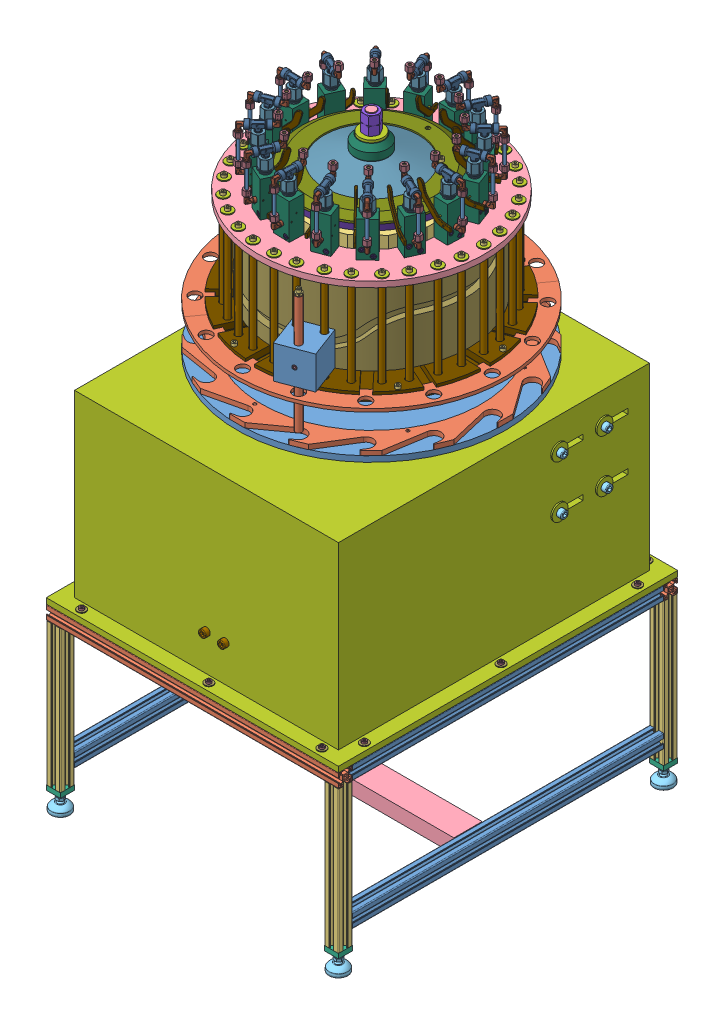
SolidWorks assembly Assieme_FINALE, configuration Default. Lengths in mm. (continued)
Components (placement in the parent): (continued)
- assieme parte rotante-2: assieme parte rotante [Default] at (-160.1634 623.9178 -718.4345) x (0 1 0) z (-0.527591 0 0.849499) size (749.63 778.63 778.63) (continued)
  - AssiemeValvola-16: AssiemeValvola [Default] at (515.3257 153.2338 311.5106) x (0 -0.793353 0.608761) z (0 0.608761 0.793353) size (90.26 138.63 38) (continued)
    - Raccordo a L-2: Raccordo a L [Default] at (30 0 0) x (0 1 0) z (0 0 -1) size (28.34 25.51 14.01)
      - 1809_06_10_01-1: 1809_06_10_01 [Default] at origin size (22.49 23 10)
      - 1809_06_10_02-1: 1809_06_10_02 [Default] at origin size (6.5 8.5 8.5)
      - 1809_06_10_03-1: 1809_06_10_03 [Default] at origin size (11.02 15.01 14.01)
    - TappoChiusura-1: TappoChiusura [Default] at (0 -32 0) x (0 -1 0) z (0 0 1) size (38.28 26.74 26.74)
    - CorpoValvola-1: CorpoValvola [Default] at (-15 -115.2824 0) size (30 75 34)
    - Raccordo a L-3: Raccordo a L [Default] at (-30 -88.2824 0) x (0 1 0) z (0 0 1) size (28.34 25.51 14.01)
      - 1809_06_10_01-1: 1809_06_10_01 [Default] at origin size (22.49 23 10)
      - 1809_06_10_02-1: 1809_06_10_02 [Default] at origin size (6.5 8.5 8.5)
      - 1809_06_10_03-1: 1809_06_10_03 [Default] at origin size (11.02 15.01 14.01)
    - Spina_3x38-1: Spina_3x38 [Default] at (0 -68.2824 -21) x (-1 0 0) z (0 0 1) size (3 3 38)
    - Spina_3x38-2: Spina_3x38 [Default] at (-10 -80.2824 -21) x (0.996193 0.087174 0) z (0 0 1) size (3 3 38)
    - M5 40mm-3: M5 40mm [ISO 4762 M5 x 40 - 40N] at (-14.6 -108.7824 9) size (45 8.5 8.5)
    - M5 40mm-2: M5 40mm [ISO 4762 M5 x 40 - 40N] at (-14.6 -96.7824 -9) size (45 8.5 8.5)
    - LevaValvola-1: LevaValvola [Default] at (-24.507 -86.571 -17) x (0.996193 0.087174 0) z (0 0 1) size (77.55 60.2 4)
    - Tubo-1: Tubo [Default] at (-30 -15.9665 0) x (1 0 0) z (0 -1 0) size (6 6 56.4)
  - Disco alimentazione guarnizione fi24.4-1: Disco alimentazione guarnizione fi24.4 [Default] at (198.0433 18.3637 415) x (0 0.065403 0.997859) z (-1 0 0) size (570 285 7.35)
  - Disco alimentazione guarnizione fi24.4-2: Disco alimentazione guarnizione fi24.4 [Default] at (198.0433 18.3637 415) x (0 -0.065403 -0.997859) z (-1 0 0) size (570 285 7.35)
  - m6 12mm-1: m6 12mm [ISO 4762 M6 x 12 - 12N] at (210.0433 200.6849 574.8914) x (-1 0 0) z (0 0.793353 -0.608761) size (18 10 10)
  - m6 12mm-7: m6 12mm [ISO 4762 M6 x 12 - 12N] at (210.0433 260.3445 399.1397) x (-1 0 0) z (0 0.793353 -0.608761) size (18 10 10)
  - m6 12mm-8: m6 12mm [ISO 4762 M6 x 12 - 12N] at (210.0433 96.3128 185.3694) x (-1 0 0) z (0 0.793353 -0.608761) size (18 10 10)
  - m6 12mm-9: m6 12mm [ISO 4762 M6 x 12 - 12N] at (210.0433 -59.5854 644.6306) x (-1 0 0) z (0 -0.793353 -0.608761) size (18 10 10)
  - m6 12mm-10: m6 12mm [ISO 4762 M6 x 12 - 12N] at (210.0433 -223.6171 430.8603) x (-1 0 0) z (0 -0.793353 -0.608761) size (18 10 10)
  - m6 12mm-11: m6 12mm [ISO 4762 M6 x 12 - 12N] at (210.0433 -163.9575 255.1086) x (-1 0 0) z (0 0.793353 -0.608761) size (18 10 10)
- assieme parte fissa-1: assieme parte fissa [Default] at (-1179.2365 708.9757 -309.8267) x (0 -1 0) z (1 0 0) size (784.52 415.1 415.07)
  - AlberoPortaCamme-1: AlberoPortaCamme [Default] at (-462.1354 65.7544 784.523) size (784.52 50 50)
  - linguetta_uni_6604_a_14x9x150-1: linguetta_uni_6604_a_14x9x150 [Default] at (-282.1354 65.7544 802.023) x (1 0 0) z (0 -1 0) size (150 9 14)
  - linguetta_uni_6604_a_8x7x50-1: linguetta_uni_6604_a_8x7x50 [Default] at (-397.1354 65.7544 802.523) x (1 0 0) z (0 1 0) size (50 7 8)
  - linguetta_uni_6604_a_8x7x50-2: linguetta_uni_6604_a_8x7x50 [Default] at (-397.1354 65.7544 766.523) x (1 0 0) z (0 -1 0) size (50 7 8)
  - rondella 20d 50D 5mm-1: rondella 20d 50D 5mm [Default] at (-417.3639 65.7544 784.523) x (0 0 1) z (-1 0 0) size (50 50 5)
  - dado M20-3: dado M20 [ISO - 4034 - M20 - N] at (-441.3639 65.7544 784.523) x (0 -1 0) z (1 0 0) size (30 34.64 19)
  - dado M20-2: dado M20 [ISO - 4034 - M20 - N] at (-422.3639 65.7544 784.523) x (0 -1 0) z (1 0 0) size (30 34.64 19)
  - seger 47-11: seger 47 [B27.7M - 3AM1-50] at (292.1646 65.7544 784.523) x (0 0 -1) z (1 0 0) size (54.93 58.5 1.6)
  - seger 47-12: seger 47 [B27.7M - 3AM1-50] at (272.8646 65.7544 784.523) x (0 0 1) z (-1 0 0) size (54.93 58.5 1.6)
  - seger 47-13: seger 47 [B27.7M - 3AM1-50] at (-120.5354 65.7544 784.523) x (0 0 -1) z (1 0 0) size (54.93 58.5 1.6)
  - seger 47-14: seger 47 [B27.7M - 3AM1-50] at (-104.4354 65.7544 784.523) x (0 0 1) z (-1 0 0) size (54.93 58.5 1.6)
  - seger 45mm-2: seger 45mm [seger 45mm] at (-289.9354 65.7544 784.523) x (0 1 0) z (-1 0 0) size (52.13 56.09 2.8)
  - seger 40mm-3: seger 40mm [B27.8M - 3DM1-40] at (-342.1354 65.7544 784.523) x (0 -1 0) z (1 0 0) size (46.31 50.39 2.8)
  - camma-1: camma [Default] at (-135.1932 65.7544 784.523) x (0 1 0) z (0 0 1) size (415.1 160.05 415.07)
  - SKF - 6010 - 18,DE,NC,18_68-1: SKF - 6010 - 18,DE,NC,18_68 [SKF - 6010 - 18,DE,NC,18_68] at (282.5646 65.7544 784.523) size (16 80 80)
  - SKF - 6010 - 18,DE,NC,18_68-2: SKF - 6010 - 18,DE,NC,18_68 [SKF - 6010 - 18,DE,NC,18_68] at (-112.5354 65.7544 784.523) size (16 80 80)
  - assieme molla e distributore-2: assieme molla e distributore [Default] at (-388.2308 60.5069 994.523) x (0 -1 0) z (0 0 -1) size (295 75.23 295)
    - molla a tazza-1: molla a tazza [Default] at (-5.2475 5.9046 210) size (200 27.84 200)
    - flangia copertura molla-1: flangia copertura molla [Default] at (-5.2475 11.1331 210) size (70 28.5 70)
    - distributore_fisso-1: distributore_fisso [Default] at (-5.2475 -46.0954 210) x (1 0 0) z (0 1 0) size (295 295 47)
    - delring_distributore_fisso-1: delring_distributore_fisso [Default] at (-5.2475 -46.0954 210) x (0 0 1) z (0 1 0) size (295 295 12)
    - O-ring 12.5x1.8-A-ISO 3601-1-2: O-ring 12.5x1.8-A-ISO 3601-1 [O-ring 12.5x1.8-A-ISO 3601-1] at (-125.2475 -33.1954 210) x (0.868916 0 -0.49496) z (0 1 0) size (16.1 16.1 1.8)
    - M6 16mm-6: M6 16mm [ISO 4762 M6 x 16 - 16N] at (-79.4937 -15.0954 135.7538) x (0 -1 0) z (0 0 1) size (22 10 10)
    - M6 16mm-7: M6 16mm [ISO 4762 M6 x 16 - 16N] at (-79.4937 -15.0954 284.2462) x (0 -1 0) z (1 0 0) size (22 10 10)
    - M6 16mm-8: M6 16mm [ISO 4762 M6 x 16 - 16N] at (68.9987 -15.0954 284.2462) x (0 -1 0) z (0 0 -1) size (22 10 10)
    - M6 16mm-9: M6 16mm [ISO 4762 M6 x 16 - 16N] at (68.9987 -15.0954 135.7538) x (0 -1 0) z (-1 0 0) size (22 10 10)
- assieme_carrello_movimento-1: assieme_carrello_movimento [Default] at (-297.3118 806.1401 -150.1164) x (0.935708 0 -0.352776) z (0 1 0) size (70 82 262.71)
  - carello movimento alternativo-1: carello movimento alternativo [Default] at (-11.6011 0.1165 35) size (70 70 70)
  - tubo_carello-1: tubo_carello [Default] at (-11.6011 -19.6699 70) x (0 -1 0) z (0 0 1) size (14 14 250)
  - raccordo dritto-1: raccordo dritto [Default] at (-11.6011 -19.6699 191.1) x (-1 0 0) z (0 1 0) size (14 16.61 13)
  - grano M8 12mm p-1: grano M8 12mm p [ISO 4026 - M8 x 12-N] at (-11.6011 -34.6699 70) x (0 1 0) z (0.714486 0 -0.69965) size (12 8 8)
  - SKF_KR_19_PPA-1: SKF_KR_19_PPA [Default] at (-11.6011 47.3301 70) x (0 -1 0) z (-0.951057 0 0.309017) size (32 19 19)
Mates (geometry in assembly coordinates):
- Parallelo2: parallel aligned: plane of SupportoBase_Totale-2 through (4.0127 -14.4529 -3.9361) normal (0 1 0)
- Perpendicolare1: perpendicular: plane of SupportoBase_Totale-2 through (4.0127 -14.4529 -3.9361) normal (0 1 0)
- Parallelo4: parallel aligned: plane of SupportoBase_Totale-2 through (4.0127 -14.4529 -3.9361) normal (0 0 1)
- Coincidente5: coincident anti-aligned: plane of SupportoBase_Totale-2/assieme_base-1/Supporto di Base per macchina-1 through (-154.7135 275.9611 -15.5811) normal (-1 0 0); plane of motoriduttore-1 through (-154.7135 275.9611 -1137.0941) normal (1 0 0)
- Tangente1: tangent anti-aligned: plane of SupportoBase_Totale-2/assieme_base-1/Supporto di Base per macchina-1 through (-93.2286 597.9611 -659.5811) normal (0 1 0); cylinder of motoriduttore-1 through (-154.7135 603.4611 -608.0941) axis (-1 0 0) radius 5.5
- Concentrico1: concentric anti-aligned: cylinder of motoriduttore-1 through (-267.2135 442.7547 -555.0941) axis (0 1 0) radius 15; cylinder of Assieme_Riduttore-1/AlberoRiduttore-1 through (-267.2135 379.4375 -555.0941) axis (0 -1 0) radius 12.5
- Coincidente9: coincident anti-aligned: plane of motoriduttore-1 through (-164.7135 602.1811 -1137.0941) normal (0 1 0); plane of Assieme_Riduttore-1/Rondella di fermo-2 through (-267.2135 602.1811 -555.0941) normal (0 -1 0)
- Coincidente12: coincident anti-aligned: plane of M10 50mm-1 through (-131.7135 606.5159 -520.4879) normal (-1 0 0); plane of plain washer xlarge grade c_iso-1 through (-131.7135 596.9697 -497.3823) normal (1 0 0)
- Concentrico4: concentric aligned: cylinder of M10 50mm-1 through (-89.9635 603.4611 -513.0941) axis (1 0 0) radius 5; cylinder of plain washer xlarge grade c_iso-1 through (-99.7885 603.4611 -513.0941) axis (1 0 0) radius 5.5
- Coincidente13: coincident anti-aligned: plane of M10 50mm-2 through (-131.7135 484.4611 -513.0941) normal (-1 0 0); plane of plain washer xlarge grade c_iso-2 through (-131.7135 475.4611 -513.0941) normal (1 0 0)
- Concentrico5: concentric aligned: cylinder of M10 50mm-2 through (-89.9635 492.4611 -513.0941) axis (1 0 0) radius 5; cylinder of plain washer xlarge grade c_iso-2 through (-99.7885 492.4611 -513.0941) axis (1 0 0) radius 5.5
- Coincidente14: coincident anti-aligned: plane of M10 50mm-5 through (-131.7135 595.4611 -608.0941) normal (-1 0 0); plane of plain washer xlarge grade c_iso-4 through (-131.7135 586.4611 -608.0941) normal (1 0 0)
- Concentrico6: concentric aligned: cylinder of M10 50mm-5 through (-89.9635 603.4611 -608.0941) axis (1 0 0) radius 5; cylinder of plain washer xlarge grade c_iso-4 through (-99.7885 603.4611 -608.0941) axis (1 0 0) radius 5.5
- Coincidente15: coincident anti-aligned: plane of M10 50mm-4 through (-131.7135 484.4611 -608.0941) normal (-1 0 0); plane of plain washer xlarge grade c_iso-3 through (-131.7135 475.4611 -608.0941) normal (1 0 0)
- Concentrico7: concentric aligned: cylinder of M10 50mm-4 through (-89.9635 492.4611 -608.0941) axis (1 0 0) radius 5; cylinder of plain washer xlarge grade c_iso-3 through (-99.7885 492.4611 -608.0941) axis (1 0 0) radius 5.5
- Concentrico8: concentric anti-aligned: cylinder of motoriduttore-1 through (-154.7135 603.4611 -608.0941) axis (-1 0 0) radius 5.5; cylinder of M10 50mm-5 through (-89.9635 603.4611 -608.0941) axis (1 0 0) radius 5
- Coincidente16: coincident anti-aligned: plane of SupportoBase_Totale-2/assieme_base-1/Supporto di Base per macchina-1 through (-134.7135 287.9611 -15.5811) normal (1 0 0); plane of plain washer xlarge grade c_iso-4 through (-134.7135 597.9611 -608.0941) normal (-1 0 0)
- Concentrico9: concentric anti-aligned: cylinder of motoriduttore-1 through (-154.7135 603.4611 -513.0941) axis (-1 0 0) radius 5.5; cylinder of M10 50mm-1 through (-89.9635 603.4611 -513.0941) axis (1 0 0) radius 5
- Coincidente17: coincident anti-aligned: plane of SupportoBase_Totale-2/assieme_base-1/Supporto di Base per macchina-1 through (-134.7135 287.9611 -15.5811) normal (1 0 0); plane of plain washer xlarge grade c_iso-1 through (-134.7135 601.3609 -508.0109) normal (-1 0 0)
- Coincidente18: coincident anti-aligned: plane of SupportoBase_Totale-2/assieme_base-1/Supporto di Base per macchina-1 through (-134.7135 287.9611 -15.5811) normal (1 0 0); plane of plain washer xlarge grade c_iso-3 through (-134.7135 486.9611 -608.0941) normal (-1 0 0)
- Concentrico10: concentric aligned: circle of motoriduttore-1; cylinder of M10 50mm-4 through (-89.9635 492.4611 -608.0941) axis (1 0 0) radius 5
- Coincidente19: coincident anti-aligned: plane of SupportoBase_Totale-2/assieme_base-1/Supporto di Base per macchina-1 through (-134.7135 287.9611 -15.5811) normal (1 0 0); plane of plain washer xlarge grade c_iso-2 through (-134.7135 486.9611 -513.0941) normal (-1 0 0)
- Concentrico11: concentric aligned: circle of motoriduttore-1; cylinder of M10 50mm-2 through (-89.9635 492.4611 -513.0941) axis (1 0 0) radius 5
- Concentrico12: concentric anti-aligned: cylinder of M10 50mm-4 through (-89.9635 492.4611 -608.0941) axis (1 0 0) radius 5; cylinder of hex nut style 2 gradeab_iso-7 through (-164.7135 492.4611 -608.0941) axis (-1 0 0) radius 4.25
- Coincidente20: coincident anti-aligned: plane of motoriduttore-1 through (-164.7135 275.9611 -1137.0941) normal (-1 0 0); plane of hex nut style 2 gradeab_iso-7 through (-164.7135 501.6987 -608.0941) normal (1 0 0)
- Concentrico13: concentric anti-aligned: cylinder of M10 50mm-5 through (-89.9635 603.4611 -608.0941) axis (1 0 0) radius 5; cylinder of hex nut style 2 gradeab_iso-5 through (-164.7135 603.4611 -608.0941) axis (-1 0 0) radius 4.25
- Coincidente21: coincident aligned: plane of motoriduttore-1 through (-164.7135 275.9611 -1137.0941) normal (-1 0 0); circle of hex nut style 2 gradeab_iso-1
- Concentrico14: concentric anti-aligned: cylinder of M10 50mm-1 through (-89.9635 603.4611 -513.0941) axis (1 0 0) radius 5; cylinder of hex nut style 2 gradeab_iso-8 through (-164.7135 603.4611 -513.0941) axis (-1 0 0) radius 4.25
- Coincidente22: coincident anti-aligned: plane of motoriduttore-1 through (-164.7135 275.9611 -1137.0941) normal (-1 0 0); plane of hex nut style 2 gradeab_iso-8 through (-164.7135 612.6987 -513.0941) normal (1 0 0)
- Concentrico15: concentric anti-aligned: cylinder of M10 50mm-2 through (-89.9635 492.4611 -513.0941) axis (1 0 0) radius 5; cylinder of hex nut style 2 gradeab_iso-6 through (-164.7135 492.4611 -513.0941) axis (-1 0 0) radius 4.25
- Coincidente23: coincident anti-aligned: plane of motoriduttore-1 through (-164.7135 275.9611 -1137.0941) normal (-1 0 0); plane of hex nut style 2 gradeab_iso-6 through (-164.7135 501.6987 -513.0941) normal (1 0 0)
- Concentrico164: concentric anti-aligned: cylinder of SupportoBase_Totale-2/assieme_base-1/Traversa di blocco albero-1 through (-394.7135 362.1119 -360.5811) axis (0 1 0) radius 5.25; cylinder of assieme parte fissa-1/AlberoPortaCamme-1 through (-394.7135 386.9611 -360.5811) axis (0 -1 0) radius 4.5
- Coincidente26: coincident anti-aligned: plane of SupportoBase_Totale-2/assieme_base-1/Traversa di blocco albero-1 through (-427.2135 386.9611 -53.5811) normal (0 1 0); plane of assieme parte fissa-1/AlberoPortaCamme-1 through (-394.7135 386.9611 -400.5811) normal (0 -1 0)
- Concentrico1651: concentric aligned: cylinder of SupportoBase_Totale-2/assieme_base-1/Traversa di blocco albero-1 through (-394.7135 362.1119 -360.5811) axis (0 1 0) radius 5.25; cylinder of rondella M8-1 through (-394.7135 374.9611 -360.5811) axis (0 1 0) radius 4.65
- Coincidente271: coincident anti-aligned: plane of SupportoBase_Totale-2/assieme_base-1/Traversa di blocco albero-1 through (-427.2135 376.9611 -53.5811) normal (0 -1 0); plane of rondella M8-1 through (-394.7135 376.9611 -360.5811) normal (0 1 0)
- Concentrico1661: concentric aligned: cylinder of SupportoBase_Totale-2/assieme_base-1/Traversa di blocco albero-1 through (-394.7135 362.1119 -390.5811) axis (0 1 0) radius 5.25; cylinder of rondella M8-2 through (-394.7135 374.9611 -390.5811) axis (0 1 0) radius 4.65
- Coincidente281: coincident anti-aligned: plane of SupportoBase_Totale-2/assieme_base-1/Traversa di blocco albero-1 through (-427.2135 376.9611 -53.5811) normal (0 -1 0); plane of rondella M8-2 through (-394.7135 376.9611 -390.5811) normal (0 1 0)
- Coincidente29: coincident aligned: plane of rondella M8-1 through (-394.7135 376.9611 -360.5811) normal (-1 0 0); plane of rondella M8-2 through (-394.7135 376.9611 -390.5811) normal (-1 0 0)
- Concentrico16621: concentric anti-aligned: cylinder of SupportoBase_Totale-2/assieme_base-1/Traversa di blocco albero-1 through (-394.7135 362.1119 -390.5811) axis (0 1 0) radius 5.25; cylinder of M8 25 mm-1 through (-394.7135 337.2111 -390.5811) axis (0 -1 0) radius 6.5
- Coincidente2821: coincident anti-aligned: plane of SupportoBase_Totale-2/assieme_base-1/Traversa di blocco albero-1 through (-427.2135 376.9611 -53.5811) normal (0 -1 0); plane of M8 25 mm-1 through (-400.3427 376.9611 -387.3311) normal (0 1 0)
- Concentrico16631: concentric anti-aligned: cylinder of rondella M8-1 through (-394.7135 374.9611 -360.5811) axis (0 1 0) radius 4.65; cylinder of M8 25 mm-2 through (-394.7135 335.2111 -360.5811) axis (0 -1 0) radius 6.5
- Coincidente284: coincident anti-aligned: plane of rondella M8-1 through (-394.7135 374.9611 -360.5811) normal (0 -1 0); plane of M8 25 mm-2 through (-389.0844 374.9611 -363.8311) normal (0 1 0)
- Coincidente285: coincident aligned: plane of M8 25 mm-1 through (-391.666 372.9611 -388.8216) normal (-1 0 0); plane of M8 25 mm-2 through (-391.666 370.9611 -362.3406) normal (-1 0 0)
- Concentrico16632: concentric aligned: cylinder of assieme parte rotante-1/asta scorrimento carello-15 through (-613.1413 1023.9611 -329.7302) axis (0 -1 0) radius 6; cylinder of assieme_carrello_movimento-1/carello movimento alternativo-1 through (-294.876 911.1401 -175.9678) axis (0 -1 0) radius 7
- Concentrico16635: concentric anti-aligned: cylinder of assieme parte rotante-1/asta scorrimento carello-30 through (-617.9018 798.9611 -375.4832) axis (0 1 0) radius 6; cylinder of assieme_carrello_movimento-1/carello movimento alternativo-1 through (-337.9186 911.1401 -159.7401) axis (0 -1 0) radius 7
- Concentrico16636: concentric aligned: cylinder of assieme parte rotante-1/asta scorrimento carello-16 through (-614.0609 1023.9611 -416.8091) axis (0 -1 0) radius 6; cylinder of assieme_carrello_movimento-2/carello movimento alternativo-1 through (-815.5741 1126.98 -443.8548) axis (0.792505 0.608914 0.03405) radius 7
- Concentrico16637: concentric anti-aligned: cylinder of assieme parte rotante-1/asta scorrimento carello-31 through (-600.95 798.9611 -460.9011) axis (0 1 0) radius 6; cylinder of assieme_carrello_movimento-2/carello movimento alternativo-1 through (-808.6117 1115.4588 -399.8685) axis (0.792505 0.608914 0.03405) radius 7
- Tangente3: tangent: face of ?; circle of ?
- Concentrico16638: concentric aligned: cylinder of assieme_carrello_movimento-3/carello movimento alternativo-1 through (-942.7141 999.5638 -329.9276) axis (0.116747 -0.965603 -0.232337) radius 7; cylinder of assieme parte rotante-1/asta scorrimento carello-17 through (-581.5867 1023.9611 -497.6114) axis (0 -1 0) radius 6
- Concentrico16640: concentric anti-aligned: cylinder of assieme parte rotante-1/asta scorrimento carello-32 through (-552.6006 798.9611 -533.3298) axis (0 1 0) radius 6; cylinder of assieme_carrello_movimento-3/carello movimento alternativo-1 through (-913.7159 1011.1934 -363.6893) axis (0.116747 -0.965603 -0.232337) radius 7
- Concentrico16641: concentric aligned: cylinder of assieme parte rotante-1/asta scorrimento carello-1 through (-520.6629 1023.9611 -559.8357) axis (0 -1 0) radius 6; cylinder of assieme_carrello_movimento-4/carello movimento alternativo-1 through (-1014.341 1005.0328 -455.3759) axis (-0.04516 -0.99458 -0.093653) radius 7
- Concentrico16642: concentric anti-aligned: cylinder of assieme parte rotante-1/asta scorrimento carello-2 through (-480.2144 798.9611 -581.7427) axis (0 1 0) radius 6; cylinder of assieme_carrello_movimento-4/carello movimento alternativo-1 through (-973.9216 1005.2653 -477.3352) axis (-0.04516 -0.99458 -0.093653) radius 7
- Tangente5: tangent: plane of assieme parte fissa-1/camma-1 through (-382.97 980.6111 -351.2489) normal (0 -1 0); circle of assieme_carrello_movimento-4/SKF_KR_19_PPA-1
- Tangente6: tangent: plane of assieme parte fissa-1/camma-1 through (-382.97 980.6111 -351.2489) normal (0 -1 0); circle of assieme_carrello_movimento-3/SKF_KR_19_PPA-1
- Concentrico16643: concentric anti-aligned: cylinder of assieme parte rotante-1/asta scorrimento carello-18 through (-394.8114 798.9611 -598.7693) axis (0 1 0) radius 6; cylinder of assieme_carrello_movimento-5/carello movimento alternativo-1 through (-942.937 1344.8131 -503.9041) axis (0.392311 0.281014 0.875856) radius 7
- Concentrico16644: concentric aligned: cylinder of assieme parte rotante-1/asta scorrimento carello-3 through (-440.5644 1023.9611 -594.0089) axis (0 -1 0) radius 6; cylinder of assieme_carrello_movimento-5/carello movimento alternativo-1 through (-900.7589 1335.8317 -519.9148) axis (0.392311 0.281014 0.875856) radius 7
- Tangente7: tangent: plane of assieme parte fissa-1/camma-1 through (-382.97 980.6111 -351.2489) normal (0 -1 0); circle of assieme_carrello_movimento-5/SKF_KR_19_PPA-1
- Concentrico16645: concentric aligned: cylinder of assieme parte rotante-1/asta scorrimento carello-4 through (-353.4855 1023.9611 -594.9284) axis (0 -1 0) radius 6; cylinder of assieme_carrello_movimento-8/carello movimento alternativo-1 through (-969.7947 1516.1419 -621.2277) axis (0 -1 0) radius 7
- Concentrico16646: concentric aligned: cylinder of assieme parte rotante-1/asta scorrimento carello-5 through (-272.6832 1023.9611 -562.4543) axis (0 -1 0) radius 6; cylinder of assieme_carrello_movimento-7/carello movimento alternativo-1 through (-1060.7855 1489.752 -716.9097) axis (0 -1 0) radius 7
- Concentrico16647: concentric anti-aligned: cylinder of assieme parte rotante-1/asta scorrimento carello-19 through (-309.3935 798.9611 -581.8176) axis (0 1 0) radius 6; cylinder of assieme_carrello_movimento-8/carello movimento alternativo-1 through (-925.7026 1516.1419 -608.1168) axis (0 -1 0) radius 7
- Concentrico16648: concentric aligned: cylinder of assieme parte fissa-1/AlberoPortaCamme-1 through (-394.7135 1275.1556 -375.5811) axis (0 1 0) radius 25; cylinder of assieme parte rotante-2/albero rotazione piatti-1 through (-394.7135 684.3308 -375.5811) axis (0 1 0) radius 35
- Coincidente2822: coincident anti-aligned: plane of SupportoBase_Totale-2/assieme_base-1/canotto di supporto-1 through (-394.7135 673.9611 -375.5811) normal (0 1 0); plane of assieme parte rotante-2/SKF - 6020 - 20,DE,NC,20_68-2 through (-363.7996 673.9611 -327.0983) normal (0 -1 0)
- Concentrico16650: concentric aligned: cylinder of SupportoBase_Totale-2/assieme_base-1/canotto di supporto-1 through (-394.7135 587.1745 -375.5811) axis (0 1 0) radius 67.5; cylinder of assieme parte fissa-1/AlberoPortaCamme-1 through (-394.7135 1275.1556 -375.5811) axis (0 1 0) radius 25
- Concentrico16651: concentric anti-aligned: cylinder of assieme parte rotante-2/asta scorrimento carello-23 through (-337.9186 798.9611 -159.7401) axis (0 1 0) radius 6; cylinder of assieme_carrello_movimento-1/carello movimento alternativo-1 through (-337.9186 911.1401 -159.7401) axis (0 -1 0) radius 7
- Concentrico16652: concentric aligned: cylinder of assieme parte rotante-2/asta scorrimento carello-8 through (-294.876 1023.9611 -175.9678) axis (0 -1 0) radius 6; cylinder of assieme_carrello_movimento-1/carello movimento alternativo-1 through (-294.876 911.1401 -175.9678) axis (0 -1 0) radius 7
- Tangente8: tangent: edge_curve of assieme parte fissa-1/camma-1; circle of assieme_carrello_movimento-1/SKF_KR_19_PPA-1
